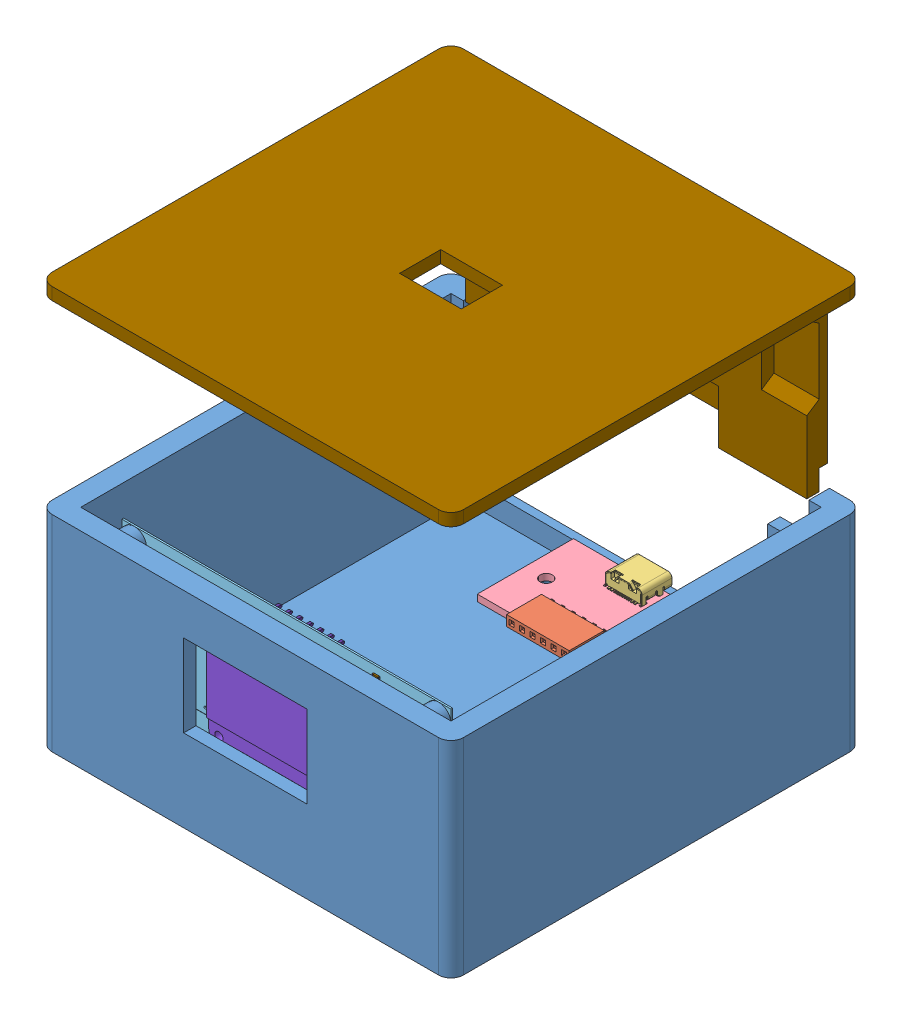
SolidWorks assembly 提醒喝水器, configuration 默认. Lengths in mm. (continued)
Components (placement in the parent): (continued)
- MainBoard-1: MainBoard [默认] at (-130.6896 -38.7345 40) size (80 40 10.66) (continued)
  - MainBoard(2)^MainBoard-1: MainBoard(2)^MainBoard [默认] at origin size (80 40 10.66) (virtual) (continued)
    - D2^MainBoard(2)_MainBoard-1: D2^MainBoard(2)_MainBoard [默认] at origin size (1.6 0.8 0.61) (virtual) (continued)
      - LED_0603-R^D2_MainBoard(2)_MainBoard-1: LED_0603-R^D2_MainBoard(2)_MainBoard [默认] at (39.878 9.398 0) x (-1 0 0) z (0 0 1) size (1.6 0.8 0.47) (virtual) (continued)
        - LED_0603-R-6878_AF0_ASM^LED_0603-R_D2_MainBoard(2)_MainBoard-1: LED_0603-R-6878_AF0_ASM^LED_0603-R_D2_MainBoard(2)_MainBoard [默认] at origin size (1.6 0.8 0.47) (virtual)
          - LED_0603-R-4157_AF0_ASM^LED_0603-R-6878_AF0_ASM_LED_0603-R_D2_MainBoard(2)_MainBoard-1: LED_0603-R-4157_AF0_ASM^LED_0603-R-6878_AF0_ASM_LED_0603-R_D2_MainBoard(2)_MainBoard [默认] at origin size (1.6 0.8 0.47) (virtual)
            - _2_1_20001^LED_0603-R-4157_AF0_ASM_LED_0603-R-6878_AF0_ASM_LED_0603-R_D2_MainBoard(2)_MainBoard-1: _2_1_20001^LED_0603-R-4157_AF0_ASM_LED_0603-R-6878_AF0_ASM_LED_0603-R_D2_MainBoard(2)_MainBoard [默认] at origin size (0.2 0.8 0.2) (virtual)
            - _5_2__1_20001^LED_0603-R-4157_AF0_ASM_LED_0603-R-6878_AF0_ASM_LED_0603-R_D2_MainBoard(2)_MainBoard-1: _5_2__1_20001^LED_0603-R-4157_AF0_ASM_LED_0603-R-6878_AF0_ASM_LED_0603-R_D2_MainBoard(2)_MainBoard [默认] at origin size (0.31 0.14 0) (virtual)
            - 4_1_200^LED_0603-R-4157_AF0_ASM_LED_0603-R-6878_AF0_ASM_LED_0603-R_D2_MainBoard(2)_MainBoard-1: 4_1_200^LED_0603-R-4157_AF0_ASM_LED_0603-R-6878_AF0_ASM_LED_0603-R_D2_MainBoard(2)_MainBoard [默认] at origin size (0.2 0.8 0.2) (virtual)
            - _5_1__1_20001^LED_0603-R-4157_AF0_ASM_LED_0603-R-6878_AF0_ASM_LED_0603-R_D2_MainBoard(2)_MainBoard-1: _5_1__1_20001^LED_0603-R-4157_AF0_ASM_LED_0603-R-6878_AF0_ASM_LED_0603-R_D2_MainBoard(2)_MainBoard [默认] at origin size (0.31 0.14 0) (virtual)
            - 1_1_2_3_4_5_6_7_8_000^LED_0603-R-4157_AF0_ASM_LED_0603-R-6878_AF0_ASM_LED_0603-R_D2_MainBoard(2)_MainBoard-1: 1_1_2_3_4_5_6_7_8_000^LED_0603-R-4157_AF0_ASM_LED_0603-R-6878_AF0_ASM_LED_0603-R_D2_MainBoard(2)_MainBoard [默认] at origin size (1.6 0.8 0.47) (virtual)
      - LED_0603______^D2_MainBoard(2)_MainBoard-1: LED_0603______^D2_MainBoard(2)_MainBoard [默认] at (39.878 9.398 0) x (1 0 0) z (0 0 1) size (1.2 0.8 0.4) (virtual)
    - D1^MainBoard(2)_MainBoard-1: D1^MainBoard(2)_MainBoard [默认] at origin size (1.5 3.4 1.5) (virtual)
      - MINI-MELF^D1_MainBoard(2)_MainBoard-1: MINI-MELF^D1_MainBoard(2)_MainBoard [默认] at (43.6879 20.0661 0) x (0 -1 0) z (0 0 1) size (3.4 1.5 1.5) (virtual)
        - MINI-MELF-5^MINI-MELF_D1_MainBoard(2)_MainBoard-1: MINI-MELF-5^MINI-MELF_D1_MainBoard(2)_MainBoard [默认] at origin size (3.4 1.5 1.5) (virtual)
        - LOGO______.____^MINI-MELF_D1_MainBoard(2)_MainBoard-1: LOGO______.____^MINI-MELF_D1_MainBoard(2)_MainBoard [默认] at (0.0006 0.0003 0.0498) x (-1 0 0) z (0 0 -1) size (0.06 0.07 0) (virtual)
    - C9^MainBoard(2)_MainBoard-1: C9^MainBoard(2)_MainBoard [默认] at origin size (1.22 2 0.52) (virtual)
      - c_0805^C9_MainBoard(2)_MainBoard-1: c_0805^C9_MainBoard(2)_MainBoard [默认] at (51.4351 17.1449 0) x (0 -1 0) z (0 0 1) size (2 1.22 0.52) (virtual)
        - C_0805-3038_AF0_ASM^c_0805_C9_MainBoard(2)_MainBoard-1: C_0805-3038_AF0_ASM^c_0805_C9_MainBoard(2)_MainBoard [默认] at origin size (2 1.22 0.52) (virtual)
          - C_0805-10418_AF0_ASM^C_0805-3038_AF0_ASM_c_0805_C9_MainBoard(2)_MainBoard-1: C_0805-10418_AF0_ASM^C_0805-3038_AF0_ASM_c_0805_C9_MainBoard(2)_MainBoard [默认] at origin size (2 1.22 0.52) (virtual)
            - 500^C_0805-10418_AF0_ASM_C_0805-3038_AF0_ASM_c_0805_C9_MainBoard(2)_MainBoard-1: 500^C_0805-10418_AF0_ASM_C_0805-3038_AF0_ASM_c_0805_C9_MainBoard(2)_MainBoard [默认] at origin size (0.3 1.22 0.52) (virtual)
            - _1_1_2_3_4_5_6_AF0^C_0805-10418_AF0_ASM_C_0805-3038_AF0_ASM_c_0805_C9_MainBoard(2)_MainBoard-1: _1_1_2_3_4_5_6_AF0^C_0805-10418_AF0_ASM_C_0805-3038_AF0_ASM_c_0805_C9_MainBoard(2)_MainBoard [默认] at origin size (1.4 1.2 0.5) (virtual)
            - 400^C_0805-10418_AF0_ASM_C_0805-3038_AF0_ASM_c_0805_C9_MainBoard(2)_MainBoard-1: 400^C_0805-10418_AF0_ASM_C_0805-3038_AF0_ASM_c_0805_C9_MainBoard(2)_MainBoard [默认] at origin size (0.3 1.22 0.52) (virtual)
    - C8^MainBoard(2)_MainBoard-1: C8^MainBoard(2)_MainBoard [默认] at origin size (2 1.22 0.52) (virtual)
      - c_0805^C8_MainBoard(2)_MainBoard-1: c_0805^C8_MainBoard(2)_MainBoard [默认] at (58.5469 12.1919 0) x (-1 0 0) z (0 0 1) size (2 1.22 0.52) (virtual)
        - C_0805-3038_AF0_ASM^c_0805_C8_MainBoard(2)_MainBoard-1: C_0805-3038_AF0_ASM^c_0805_C8_MainBoard(2)_MainBoard [默认] at origin size (2 1.22 0.52) (virtual)
          - C_0805-10418_AF0_ASM^C_0805-3038_AF0_ASM_c_0805_C8_MainBoard(2)_MainBoard-1: C_0805-10418_AF0_ASM^C_0805-3038_AF0_ASM_c_0805_C8_MainBoard(2)_MainBoard [默认] at origin size (2 1.22 0.52) (virtual)
            - 500^C_0805-10418_AF0_ASM_C_0805-3038_AF0_ASM_c_0805_C8_MainBoard(2)_MainBoard-1: 500^C_0805-10418_AF0_ASM_C_0805-3038_AF0_ASM_c_0805_C8_MainBoard(2)_MainBoard [默认] at origin size (0.3 1.22 0.52) (virtual)
            - _1_1_2_3_4_5_6_AF0^C_0805-10418_AF0_ASM_C_0805-3038_AF0_ASM_c_0805_C8_MainBoard(2)_MainBoard-1: _1_1_2_3_4_5_6_AF0^C_0805-10418_AF0_ASM_C_0805-3038_AF0_ASM_c_0805_C8_MainBoard(2)_MainBoard [默认] at origin size (1.4 1.2 0.5) (virtual)
            - 400^C_0805-10418_AF0_ASM_C_0805-3038_AF0_ASM_c_0805_C8_MainBoard(2)_MainBoard-1: 400^C_0805-10418_AF0_ASM_C_0805-3038_AF0_ASM_c_0805_C8_MainBoard(2)_MainBoard [默认] at origin size (0.3 1.22 0.52) (virtual)
    - C7^MainBoard(2)_MainBoard-1: C7^MainBoard(2)_MainBoard [默认] at origin size (1.6 0.82 0.82) (virtual)
      - c_0603^C7_MainBoard(2)_MainBoard-1: c_0603^C7_MainBoard(2)_MainBoard [默认] at (55.4989 19.431 0) x (-1 0 0) z (0 0 1) size (1.6 0.82 0.82) (virtual)
        - C_0603-7177_AF0_ASM^c_0603_C7_MainBoard(2)_MainBoard-1: C_0603-7177_AF0_ASM^c_0603_C7_MainBoard(2)_MainBoard [默认] at origin size (1.6 0.82 0.82) (virtual)
          - C_0603-683_AF0_ASM^C_0603-7177_AF0_ASM_c_0603_C7_MainBoard(2)_MainBoard-1: C_0603-683_AF0_ASM^C_0603-7177_AF0_ASM_c_0603_C7_MainBoard(2)_MainBoard [默认] at origin size (1.6 0.82 0.82) (virtual)
            - 2_1_200^C_0603-683_AF0_ASM_C_0603-7177_AF0_ASM_c_0603_C7_MainBoard(2)_MainBoard-1: 2_1_200^C_0603-683_AF0_ASM_C_0603-7177_AF0_ASM_c_0603_C7_MainBoard(2)_MainBoard [默认] at origin size (0.3 0.82 0.82) (virtual)
            - _1_1_2_3_4_5_AF0^C_0603-683_AF0_ASM_C_0603-7177_AF0_ASM_c_0603_C7_MainBoard(2)_MainBoard-1: _1_1_2_3_4_5_AF0^C_0603-683_AF0_ASM_C_0603-7177_AF0_ASM_c_0603_C7_MainBoard(2)_MainBoard [默认] at origin size (1 0.8 0.8) (virtual)
            - 3_1_200^C_0603-683_AF0_ASM_C_0603-7177_AF0_ASM_c_0603_C7_MainBoard(2)_MainBoard-1: 3_1_200^C_0603-683_AF0_ASM_C_0603-7177_AF0_ASM_c_0603_C7_MainBoard(2)_MainBoard [默认] at origin size (0.3 0.82 0.82) (virtual)
    - C6^MainBoard(2)_MainBoard-1: C6^MainBoard(2)_MainBoard [默认] at origin size (1.6 0.82 0.82) (virtual)
      - c_0603^C6_MainBoard(2)_MainBoard-1: c_0603^C6_MainBoard(2)_MainBoard [默认] at (73.6601 26.289 0) x (1 0 0) z (0 0 1) size (1.6 0.82 0.82) (virtual)
        - C_0603-7177_AF0_ASM^c_0603_C6_MainBoard(2)_MainBoard-1: C_0603-7177_AF0_ASM^c_0603_C6_MainBoard(2)_MainBoard [默认] at origin size (1.6 0.82 0.82) (virtual)
          - C_0603-683_AF0_ASM^C_0603-7177_AF0_ASM_c_0603_C6_MainBoard(2)_MainBoard-1: C_0603-683_AF0_ASM^C_0603-7177_AF0_ASM_c_0603_C6_MainBoard(2)_MainBoard [默认] at origin size (1.6 0.82 0.82) (virtual)
            - 2_1_200^C_0603-683_AF0_ASM_C_0603-7177_AF0_ASM_c_0603_C6_MainBoard(2)_MainBoard-1: 2_1_200^C_0603-683_AF0_ASM_C_0603-7177_AF0_ASM_c_0603_C6_MainBoard(2)_MainBoard [默认] at origin size (0.3 0.82 0.82) (virtual)
            - _1_1_2_3_4_5_AF0^C_0603-683_AF0_ASM_C_0603-7177_AF0_ASM_c_0603_C6_MainBoard(2)_MainBoard-1: _1_1_2_3_4_5_AF0^C_0603-683_AF0_ASM_C_0603-7177_AF0_ASM_c_0603_C6_MainBoard(2)_MainBoard [默认] at origin size (1 0.8 0.8) (virtual)
            - 3_1_200^C_0603-683_AF0_ASM_C_0603-7177_AF0_ASM_c_0603_C6_MainBoard(2)_MainBoard-1: 3_1_200^C_0603-683_AF0_ASM_C_0603-7177_AF0_ASM_c_0603_C6_MainBoard(2)_MainBoard [默认] at origin size (0.3 0.82 0.82) (virtual)
    - C5^MainBoard(2)_MainBoard-1: C5^MainBoard(2)_MainBoard [默认] at origin size (1.6 0.82 0.82) (virtual)
      - c_0603^C5_MainBoard(2)_MainBoard-1: c_0603^C5_MainBoard(2)_MainBoard [默认] at (73.6599 32.766 0) x (-1 0 0) z (0 0 1) size (1.6 0.82 0.82) (virtual)
        - C_0603-7177_AF0_ASM^c_0603_C5_MainBoard(2)_MainBoard-1: C_0603-7177_AF0_ASM^c_0603_C5_MainBoard(2)_MainBoard [默认] at origin size (1.6 0.82 0.82) (virtual)
          - C_0603-683_AF0_ASM^C_0603-7177_AF0_ASM_c_0603_C5_MainBoard(2)_MainBoard-1: C_0603-683_AF0_ASM^C_0603-7177_AF0_ASM_c_0603_C5_MainBoard(2)_MainBoard [默认] at origin size (1.6 0.82 0.82) (virtual)
            - 2_1_200^C_0603-683_AF0_ASM_C_0603-7177_AF0_ASM_c_0603_C5_MainBoard(2)_MainBoard-1: 2_1_200^C_0603-683_AF0_ASM_C_0603-7177_AF0_ASM_c_0603_C5_MainBoard(2)_MainBoard [默认] at origin size (0.3 0.82 0.82) (virtual)
            - _1_1_2_3_4_5_AF0^C_0603-683_AF0_ASM_C_0603-7177_AF0_ASM_c_0603_C5_MainBoard(2)_MainBoard-1: _1_1_2_3_4_5_AF0^C_0603-683_AF0_ASM_C_0603-7177_AF0_ASM_c_0603_C5_MainBoard(2)_MainBoard [默认] at origin size (1 0.8 0.8) (virtual)
            - 3_1_200^C_0603-683_AF0_ASM_C_0603-7177_AF0_ASM_c_0603_C5_MainBoard(2)_MainBoard-1: 3_1_200^C_0603-683_AF0_ASM_C_0603-7177_AF0_ASM_c_0603_C5_MainBoard(2)_MainBoard [默认] at origin size (0.3 0.82 0.82) (virtual)
    - C4^MainBoard(2)_MainBoard-1: C4^MainBoard(2)_MainBoard [默认] at origin size (0.82 1.6 0.82) (virtual)
      - c_0603^C4_MainBoard(2)_MainBoard-1: c_0603^C4_MainBoard(2)_MainBoard [默认] at (12.192 7.6201 0) x (0 1 0) z (0 0 1) size (1.6 0.82 0.82) (virtual)
        - C_0603-7177_AF0_ASM^c_0603_C4_MainBoard(2)_MainBoard-1: C_0603-7177_AF0_ASM^c_0603_C4_MainBoard(2)_MainBoard [默认] at origin size (1.6 0.82 0.82) (virtual)
          - C_0603-683_AF0_ASM^C_0603-7177_AF0_ASM_c_0603_C4_MainBoard(2)_MainBoard-1: C_0603-683_AF0_ASM^C_0603-7177_AF0_ASM_c_0603_C4_MainBoard(2)_MainBoard [默认] at origin size (1.6 0.82 0.82) (virtual)
            - 2_1_200^C_0603-683_AF0_ASM_C_0603-7177_AF0_ASM_c_0603_C4_MainBoard(2)_MainBoard-1: 2_1_200^C_0603-683_AF0_ASM_C_0603-7177_AF0_ASM_c_0603_C4_MainBoard(2)_MainBoard [默认] at origin size (0.3 0.82 0.82) (virtual)
            - _1_1_2_3_4_5_AF0^C_0603-683_AF0_ASM_C_0603-7177_AF0_ASM_c_0603_C4_MainBoard(2)_MainBoard-1: _1_1_2_3_4_5_AF0^C_0603-683_AF0_ASM_C_0603-7177_AF0_ASM_c_0603_C4_MainBoard(2)_MainBoard [默认] at origin size (1 0.8 0.8) (virtual)
            - 3_1_200^C_0603-683_AF0_ASM_C_0603-7177_AF0_ASM_c_0603_C4_MainBoard(2)_MainBoard-1: 3_1_200^C_0603-683_AF0_ASM_C_0603-7177_AF0_ASM_c_0603_C4_MainBoard(2)_MainBoard [默认] at origin size (0.3 0.82 0.82) (virtual)
    - C3^MainBoard(2)_MainBoard-1: C3^MainBoard(2)_MainBoard [默认] at origin size (0.82 1.6 0.82) (virtual)
      - c_0603^C3_MainBoard(2)_MainBoard-1: c_0603^C3_MainBoard(2)_MainBoard [默认] at (59.8169 31.3542 0) x (0 1 0) z (0 0 1) size (1.6 0.82 0.82) (virtual)
        - C_0603-7177_AF0_ASM^c_0603_C3_MainBoard(2)_MainBoard-1: C_0603-7177_AF0_ASM^c_0603_C3_MainBoard(2)_MainBoard [默认] at origin size (1.6 0.82 0.82) (virtual)
          - C_0603-683_AF0_ASM^C_0603-7177_AF0_ASM_c_0603_C3_MainBoard(2)_MainBoard-1: C_0603-683_AF0_ASM^C_0603-7177_AF0_ASM_c_0603_C3_MainBoard(2)_MainBoard [默认] at origin size (1.6 0.82 0.82) (virtual)
            - 2_1_200^C_0603-683_AF0_ASM_C_0603-7177_AF0_ASM_c_0603_C3_MainBoard(2)_MainBoard-1: 2_1_200^C_0603-683_AF0_ASM_C_0603-7177_AF0_ASM_c_0603_C3_MainBoard(2)_MainBoard [默认] at origin size (0.3 0.82 0.82) (virtual)
            - _1_1_2_3_4_5_AF0^C_0603-683_AF0_ASM_C_0603-7177_AF0_ASM_c_0603_C3_MainBoard(2)_MainBoard-1: _1_1_2_3_4_5_AF0^C_0603-683_AF0_ASM_C_0603-7177_AF0_ASM_c_0603_C3_MainBoard(2)_MainBoard [默认] at origin size (1 0.8 0.8) (virtual)
            - 3_1_200^C_0603-683_AF0_ASM_C_0603-7177_AF0_ASM_c_0603_C3_MainBoard(2)_MainBoard-1: 3_1_200^C_0603-683_AF0_ASM_C_0603-7177_AF0_ASM_c_0603_C3_MainBoard(2)_MainBoard [默认] at origin size (0.3 0.82 0.82) (virtual)
    - C2^MainBoard(2)_MainBoard-1: C2^MainBoard(2)_MainBoard [默认] at origin size (0.82 1.6 0.82) (virtual)
      - c_0603^C2_MainBoard(2)_MainBoard-1: c_0603^C2_MainBoard(2)_MainBoard [默认] at (45.3389 3.2872 0) x (0 1 0) z (0 0 1) size (1.6 0.82 0.82) (virtual)
        - C_0603-7177_AF0_ASM^c_0603_C2_MainBoard(2)_MainBoard-1: C_0603-7177_AF0_ASM^c_0603_C2_MainBoard(2)_MainBoard [默认] at origin size (1.6 0.82 0.82) (virtual)
          - C_0603-683_AF0_ASM^C_0603-7177_AF0_ASM_c_0603_C2_MainBoard(2)_MainBoard-1: C_0603-683_AF0_ASM^C_0603-7177_AF0_ASM_c_0603_C2_MainBoard(2)_MainBoard [默认] at origin size (1.6 0.82 0.82) (virtual)
            - 2_1_200^C_0603-683_AF0_ASM_C_0603-7177_AF0_ASM_c_0603_C2_MainBoard(2)_MainBoard-1: 2_1_200^C_0603-683_AF0_ASM_C_0603-7177_AF0_ASM_c_0603_C2_MainBoard(2)_MainBoard [默认] at origin size (0.3 0.82 0.82) (virtual)
            - _1_1_2_3_4_5_AF0^C_0603-683_AF0_ASM_C_0603-7177_AF0_ASM_c_0603_C2_MainBoard(2)_MainBoard-1: _1_1_2_3_4_5_AF0^C_0603-683_AF0_ASM_C_0603-7177_AF0_ASM_c_0603_C2_MainBoard(2)_MainBoard [默认] at origin size (1 0.8 0.8) (virtual)
            - 3_1_200^C_0603-683_AF0_ASM_C_0603-7177_AF0_ASM_c_0603_C2_MainBoard(2)_MainBoard-1: 3_1_200^C_0603-683_AF0_ASM_C_0603-7177_AF0_ASM_c_0603_C2_MainBoard(2)_MainBoard [默认] at origin size (0.3 0.82 0.82) (virtual)
    - C1^MainBoard(2)_MainBoard-1: C1^MainBoard(2)_MainBoard [默认] at origin size (0.82 1.6 0.82) (virtual)
      - c_0603^C1_MainBoard(2)_MainBoard-1: c_0603^C1_MainBoard(2)_MainBoard [默认] at (8.89 7.6199 0) x (0 -1 0) z (0 0 1) size (1.6 0.82 0.82) (virtual)
        - C_0603-7177_AF0_ASM^c_0603_C1_MainBoard(2)_MainBoard-1: C_0603-7177_AF0_ASM^c_0603_C1_MainBoard(2)_MainBoard [默认] at origin size (1.6 0.82 0.82) (virtual)
          - C_0603-683_AF0_ASM^C_0603-7177_AF0_ASM_c_0603_C1_MainBoard(2)_MainBoard-1: C_0603-683_AF0_ASM^C_0603-7177_AF0_ASM_c_0603_C1_MainBoard(2)_MainBoard [默认] at origin size (1.6 0.82 0.82) (virtual)
            - 2_1_200^C_0603-683_AF0_ASM_C_0603-7177_AF0_ASM_c_0603_C1_MainBoard(2)_MainBoard-1: 2_1_200^C_0603-683_AF0_ASM_C_0603-7177_AF0_ASM_c_0603_C1_MainBoard(2)_MainBoard [默认] at origin size (0.3 0.82 0.82) (virtual)
            - _1_1_2_3_4_5_AF0^C_0603-683_AF0_ASM_C_0603-7177_AF0_ASM_c_0603_C1_MainBoard(2)_MainBoard-1: _1_1_2_3_4_5_AF0^C_0603-683_AF0_ASM_C_0603-7177_AF0_ASM_c_0603_C1_MainBoard(2)_MainBoard [默认] at origin size (1 0.8 0.8) (virtual)
            - 3_1_200^C_0603-683_AF0_ASM_C_0603-7177_AF0_ASM_c_0603_C1_MainBoard(2)_MainBoard-1: 3_1_200^C_0603-683_AF0_ASM_C_0603-7177_AF0_ASM_c_0603_C1_MainBoard(2)_MainBoard [默认] at origin size (0.3 0.82 0.82) (virtual)
- OLED-1: OLED [默认] at (-75.4466 -2.0805 44.1) x (-1 0 0) z (0 0 -1) size (29.97 28.97 13.2)
  - 3D_PCB_7针SPI_2022-02-05_2022-02-05(2)^OLED-1: 3D_PCB_7针SPI_2022-02-05_2022-02-05(2)^OLED [默认] at origin size (29.97 28.97 13.2) (virtual)
    - R5(2)^3D_PCB_7针SPI_2022-02-05_2022-02-05(2)_OLED-1: R5(2)^3D_PCB_7针SPI_2022-02-05_2022-02-05(2)_OLED [默认] at (11.176 -11.303 1.6) x (0 -1 0) z (0 0 1) size (1.6 0.8 0.8) (virtual)
      - R0603^R5(2)_3D_PCB_7针SPI_2022-02-05_2022-02-05(2)_OLED-1: R0603^R5(2)_3D_PCB_7针SPI_2022-02-05_2022-02-05(2)_OLED [默认] at origin size (1.6 0.8 0.8) (virtual)
        - =_[0_1_1_5]^R0603_R5(2)_3D_PCB_7针SPI_2022-02-05_2022-02-05(2)_OLED-1: =_[0_1_1_5]^R0603_R5(2)_3D_PCB_7针SPI_2022-02-05_2022-02-05(2)_OLED [默认] at (0 0 0.4) size (1.6 0.8 0.8) (virtual)
    - R6(2)^3D_PCB_7针SPI_2022-02-05_2022-02-05(2)_OLED-1: R6(2)^3D_PCB_7针SPI_2022-02-05_2022-02-05(2)_OLED [默认] at (25.5271 -6.985 1.6) x (-1 0 0) z (0 0 1) size (1.6 0.8 0.8) (virtual)
      - R0603^R6(2)_3D_PCB_7针SPI_2022-02-05_2022-02-05(2)_OLED-1: R0603^R6(2)_3D_PCB_7针SPI_2022-02-05_2022-02-05(2)_OLED [默认] at origin size (1.6 0.8 0.8) (virtual)
        - =_[0_1_1_5]^R0603_R6(2)_3D_PCB_7针SPI_2022-02-05_2022-02-05(2)_OLED-1: =_[0_1_1_5]^R0603_R6(2)_3D_PCB_7针SPI_2022-02-05_2022-02-05(2)_OLED [默认] at (0 0 0.4) size (1.6 0.8 0.8) (virtual)
    - J1^3D_PCB_7针SPI_2022-02-05_2022-02-05(2)_OLED-1: J1^3D_PCB_7针SPI_2022-02-05_2022-02-05(2)_OLED [默认] at (15.113 -1.524 1.6) size (17.53 2.5 11.6) (virtual)
      - HDR-M-2.54_1X7^J1_3D_PCB_7针SPI_2022-02-05_2022-02-05(2)_OLED-1: HDR-M-2.54_1X7^J1_3D_PCB_7针SPI_2022-02-05_2022-02-05(2)_OLED [默认] at origin size (17.53 2.5 11.6) (virtual)
        - =_[0_1_1_10]^HDR-M-2.54_1X7_J1_3D_PCB_7针SPI_2022-02-05_2022-02-05(2)_OLED-1: =_[0_1_1_10]^HDR-M-2.54_1X7_J1_3D_PCB_7针SPI_2022-02-05_2022-02-05(2)_OLED [默认] at origin size (17.53 2.5 11.6) (virtual)
    - C5(2)^3D_PCB_7针SPI_2022-02-05_2022-02-05(2)_OLED-1: C5(2)^3D_PCB_7针SPI_2022-02-05_2022-02-05(2)_OLED [默认] at (9.271 -11.303 1.6) x (0 -1 0) z (0 0 1) size (1.6 0.8 0.8) (virtual)
      - C0603^C5(2)_3D_PCB_7针SPI_2022-02-05_2022-02-05(2)_OLED-1: C0603^C5(2)_3D_PCB_7针SPI_2022-02-05_2022-02-05(2)_OLED [默认] at origin size (1.6 0.8 0.8) (virtual)
        - =_[0_1_1_14]^C0603_C5(2)_3D_PCB_7针SPI_2022-02-05_2022-02-05(2)_OLED-1: =_[0_1_1_14]^C0603_C5(2)_3D_PCB_7针SPI_2022-02-05_2022-02-05(2)_OLED [默认] at (0 0 0.4) size (1.6 0.8 0.8) (virtual)
    - C2(2)^3D_PCB_7针SPI_2022-02-05_2022-02-05(2)_OLED-1: C2(2)^3D_PCB_7针SPI_2022-02-05_2022-02-05(2)_OLED [默认] at (24.257 -11.176 1.6) x (0 -1 0) z (0 0 1) size (1.6 0.8 0.8) (virtual)
      - C0603^C2(2)_3D_PCB_7针SPI_2022-02-05_2022-02-05(2)_OLED-1: C0603^C2(2)_3D_PCB_7针SPI_2022-02-05_2022-02-05(2)_OLED [默认] at origin size (1.6 0.8 0.8) (virtual)
        - =_[0_1_1_14]^C0603_C2(2)_3D_PCB_7针SPI_2022-02-05_2022-02-05(2)_OLED-1: =_[0_1_1_14]^C0603_C2(2)_3D_PCB_7针SPI_2022-02-05_2022-02-05(2)_OLED [默认] at (0 0 0.4) size (1.6 0.8 0.8) (virtual)
    - C3(2)^3D_PCB_7针SPI_2022-02-05_2022-02-05(2)_OLED-1: C3(2)^3D_PCB_7针SPI_2022-02-05_2022-02-05(2)_OLED [默认] at (19.558 -11.176 1.6) x (0 1 0) z (0 0 1) size (1.6 0.8 0.8) (virtual)
      - C0603^C3(2)_3D_PCB_7针SPI_2022-02-05_2022-02-05(2)_OLED-1: C0603^C3(2)_3D_PCB_7针SPI_2022-02-05_2022-02-05(2)_OLED [默认] at origin size (1.6 0.8 0.8) (virtual)
        - =_[0_1_1_14]^C0603_C3(2)_3D_PCB_7针SPI_2022-02-05_2022-02-05(2)_OLED-1: =_[0_1_1_14]^C0603_C3(2)_3D_PCB_7针SPI_2022-02-05_2022-02-05(2)_OLED [默认] at (0 0 0.4) size (1.6 0.8 0.8) (virtual)
    - C4(2)^3D_PCB_7针SPI_2022-02-05_2022-02-05(2)_OLED-1: C4(2)^3D_PCB_7针SPI_2022-02-05_2022-02-05(2)_OLED [默认] at (21.463 -11.176 1.6) x (0 1 0) z (0 0 1) size (1.6 0.8 0.8) (virtual)
      - C0603^C4(2)_3D_PCB_7针SPI_2022-02-05_2022-02-05(2)_OLED-1: C0603^C4(2)_3D_PCB_7针SPI_2022-02-05_2022-02-05(2)_OLED [默认] at origin size (1.6 0.8 0.8) (virtual)
        - =_[0_1_1_14]^C0603_C4(2)_3D_PCB_7针SPI_2022-02-05_2022-02-05(2)_OLED-1: =_[0_1_1_14]^C0603_C4(2)_3D_PCB_7针SPI_2022-02-05_2022-02-05(2)_OLED [默认] at (0 0 0.4) size (1.6 0.8 0.8) (virtual)
    - C7(2)^3D_PCB_7针SPI_2022-02-05_2022-02-05(2)_OLED-1: C7(2)^3D_PCB_7针SPI_2022-02-05_2022-02-05(2)_OLED [默认] at (18.923 -5.461 1.6) x (0 -1 0) z (0 0 1) size (1.6 0.8 0.8) (virtual)
      - C0603^C7(2)_3D_PCB_7针SPI_2022-02-05_2022-02-05(2)_OLED-1: C0603^C7(2)_3D_PCB_7针SPI_2022-02-05_2022-02-05(2)_OLED [默认] at origin size (1.6 0.8 0.8) (virtual)
        - =_[0_1_1_14]^C0603_C7(2)_3D_PCB_7针SPI_2022-02-05_2022-02-05(2)_OLED-1: =_[0_1_1_14]^C0603_C7(2)_3D_PCB_7针SPI_2022-02-05_2022-02-05(2)_OLED [默认] at (0 0 0.4) size (1.6 0.8 0.8) (virtual)
    - C1(2)^3D_PCB_7针SPI_2022-02-05_2022-02-05(2)_OLED-1: C1(2)^3D_PCB_7针SPI_2022-02-05_2022-02-05(2)_OLED [默认] at (26.5431 -11.176 1.6) x (0 -1 0) z (0 0 1) size (1.6 0.8 0.8) (virtual)
      - C0603^C1(2)_3D_PCB_7针SPI_2022-02-05_2022-02-05(2)_OLED-1: C0603^C1(2)_3D_PCB_7针SPI_2022-02-05_2022-02-05(2)_OLED [默认] at origin size (1.6 0.8 0.8) (virtual)
        - =_[0_1_1_14]^C0603_C1(2)_3D_PCB_7针SPI_2022-02-05_2022-02-05(2)_OLED-1: =_[0_1_1_14]^C0603_C1(2)_3D_PCB_7针SPI_2022-02-05_2022-02-05(2)_OLED [默认] at (0 0 0.4) size (1.6 0.8 0.8) (virtual)
    - C6(2)^3D_PCB_7针SPI_2022-02-05_2022-02-05(2)_OLED-1: C6(2)^3D_PCB_7针SPI_2022-02-05_2022-02-05(2)_OLED [默认] at (7.366 -11.303 1.6) x (0 -1 0) z (0 0 1) size (1.6 0.8 0.8) (virtual)
      - C0603^C6(2)_3D_PCB_7针SPI_2022-02-05_2022-02-05(2)_OLED-1: C0603^C6(2)_3D_PCB_7针SPI_2022-02-05_2022-02-05(2)_OLED [默认] at origin size (1.6 0.8 0.8) (virtual)
        - =_[0_1_1_14]^C0603_C6(2)_3D_PCB_7针SPI_2022-02-05_2022-02-05(2)_OLED-1: =_[0_1_1_14]^C0603_C6(2)_3D_PCB_7针SPI_2022-02-05_2022-02-05(2)_OLED [默认] at (0 0 0.4) size (1.6 0.8 0.8) (virtual)
    - U1(2)^3D_PCB_7针SPI_2022-02-05_2022-02-05(2)_OLED-1: U1(2)^3D_PCB_7针SPI_2022-02-05_2022-02-05(2)_OLED [默认] at (21.844 -5.842 1.6) x (0 -1 0) z (0 0 1) size (2.5 2.89 1.05) (virtual)
      - SOT-23-3_L2.9-W1.3-P1.90-LS2.4-BR^U1(2)_3D_PCB_7针SPI_2022-02-05_2022-02-05(2)_OLED-1: SOT-23-3_L2.9-W1.3-P1.90-LS2.4-BR^U1(2)_3D_PCB_7针SPI_2022-02-05_2022-02-05(2)_OLED [默认] at origin size (2.5 2.89 1.05) (virtual)
        - COMPOUND(2)^SOT-23-3_L2.9-W1.3-P1.90-LS2.4-BR_U1(2)_3D_PCB_7针SPI_2022-02-05_2022-02-05(2)_OLED-1: COMPOUND(2)^SOT-23-3_L2.9-W1.3-P1.90-LS2.4-BR_U1(2)_3D_PCB_7针SPI_2022-02-05_2022-02-05(2)_OLED [默认] at origin size (2.5 2.89 1.05) (virtual)
    - COMPOUND-0^3D_PCB_7针SPI_2022-02-05_2022-02-05(2)_OLED-1: COMPOUND-0^3D_PCB_7针SPI_2022-02-05_2022-02-05(2)_OLED [默认] at origin size (29.97 28.97 4.6) (virtual)
- 上盖-1: 上盖 [默认] at (-140.6896 48.7655 50) size (100 48 100)
Mates (geometry in assembly coordinates):
- 重合1: coincident anti-aligned: plane of 外壳-1 through (-103.5021 -37.2345 -36) normal (0 1 0); plane of Type-C_Ext-1/Type-C_Ext(2)^Type-C_Ext-1/Type-C_Ext PCB^Type-C_Ext(2)_Type-C_Ext-1 through (-90.7041 -37.2345 -36) normal (0 -1 0)
- 平行1: parallel aligned: plane of 外壳-1 through (-135.6896 -41.2345 -45) normal (0 0 1); plane of Type-C_Ext-1/Type-C_Ext(2)^Type-C_Ext-1/Type-C_Ext PCB^Type-C_Ext(2)_Type-C_Ext-1 through (-108.6111 -37.2345 -24.316) normal (0 0 1)
- 同心1: concentric aligned: circle of 外壳-1; circle of Type-C_Ext-1/Type-C_Ext(2)^Type-C_Ext-1/Type-C_Ext PCB^Type-C_Ext(2)_Type-C_Ext-1
- 平行2: parallel anti-aligned: plane of MainBoard-1/MainBoard(2)^MainBoard-1/Board^MainBoard(2)_MainBoard-1/Open CASCADE STEP translator 6.8 1.1.1^Board_MainBoard(2)_MainBoard-1 through (-130.6896 -38.7345 40) normal (0 0 1); plane of OLED-1/3D_PCB_7针SPI_2022-02-05_2022-02-05(2)^OLED-1/COMPOUND-0^3D_PCB_7针SPI_2022-02-05_2022-02-05(2)_OLED-1 through (-90.5084 -16.8409 42.5) normal (0 0 -1)
- 平行5: parallel aligned: plane of 外壳-1 through (-137.6896 3.7655 -50) normal (0 0 -1); plane of MainBoard-1/MainBoard(2)^MainBoard-1/Board^MainBoard(2)_MainBoard-1/Open CASCADE STEP translator 6.8 1.1.1^Board_MainBoard(2)_MainBoard-1 through (-130.6896 -38.7345 39.5885) normal (0 0 -1)
- 平行7: parallel aligned: plane of 外壳-1 through (-140.6896 -41.2345 50) normal (0 1 0); plane of MainBoard-1/MainBoard(2)^MainBoard-1/Board^MainBoard(2)_MainBoard-1/Open CASCADE STEP translator 6.8 1.1.1^Board_MainBoard(2)_MainBoard-1 through (-130.6896 1.2655 39.5885) normal (0 1 0)
- 重合13: coincident anti-aligned: plane of MainBoard-1/MainBoard(2)^MainBoard-1/Board^MainBoard(2)_MainBoard-1/Open CASCADE STEP translator 6.8 1.1.1^Board_MainBoard(2)_MainBoard-1 through (-130.6896 -38.7345 40) normal (0 0 1); plane of OLED-1/3D_PCB_7针SPI_2022-02-05_2022-02-05(2)^OLED-1/J1^3D_PCB_7针SPI_2022-02-05_2022-02-05(2)_OLED-1/HDR-M-2.54_1X7^J1_3D_PCB_7针SPI_2022-02-05_2022-02-05(2)_OLED-1/=_[0_1_1_10]^HDR-M-2.54_1X7_J1_3D_PCB_7针SPI_2022-02-05_2022-02-05(2)_OLED-1 through (-90.5596 -3.6045 40) normal (0 0 -1)
- 同心2: concentric anti-aligned: circle of 外壳-1; circle of MainBoard-1/MainBoard(2)^MainBoard-1/Board^MainBoard(2)_MainBoard-1/Open CASCADE STEP translator 6.8 1.1.1^Board_MainBoard(2)_MainBoard-1
- 重合14: coincident anti-aligned: plane of 外壳-1 through (-53.6896 -1.7345 40) normal (0 0 -1); plane of MainBoard-1/MainBoard(2)^MainBoard-1/Board^MainBoard(2)_MainBoard-1/Open CASCADE STEP translator 6.8 1.1.1^Board_MainBoard(2)_MainBoard-1 through (-130.6896 -38.7345 40) normal (0 0 1)
- 相切2: tangent: circle of MainBoard-1/MainBoard(2)^MainBoard-1/Board^MainBoard(2)_MainBoard-1/Open CASCADE STEP translator 6.8 1.1.1^Board_MainBoard(2)_MainBoard-1; plane of OLED-1/3D_PCB_7针SPI_2022-02-05_2022-02-05(2)^OLED-1/J1^3D_PCB_7针SPI_2022-02-05_2022-02-05(2)_OLED-1/HDR-M-2.54_1X7^J1_3D_PCB_7针SPI_2022-02-05_2022-02-05(2)_OLED-1/=_[0_1_1_10]^HDR-M-2.54_1X7_J1_3D_PCB_7针SPI_2022-02-05_2022-02-05(2)_OLED-1 through (-82.6196 -3.2845 45.3) normal (0 1 0)
- 平行8: parallel aligned: plane of MainBoard-1/MainBoard(2)^MainBoard-1/Board^MainBoard(2)_MainBoard-1/Open CASCADE STEP translator 6.8 1.1.1^Board_MainBoard(2)_MainBoard-1 through (-130.6896 1.2655 39.5885) normal (0 1 0); plane of OLED-1/3D_PCB_7针SPI_2022-02-05_2022-02-05(2)^OLED-1/J1^3D_PCB_7针SPI_2022-02-05_2022-02-05(2)_OLED-1/HDR-M-2.54_1X7^J1_3D_PCB_7针SPI_2022-02-05_2022-02-05(2)_OLED-1/=_[0_1_1_10]^HDR-M-2.54_1X7_J1_3D_PCB_7针SPI_2022-02-05_2022-02-05(2)_OLED-1 through (-82.6196 -3.2845 45.3) normal (0 1 0)
- 相切4: tangent: circle of MainBoard-1/MainBoard(2)^MainBoard-1/Board^MainBoard(2)_MainBoard-1/Open CASCADE STEP translator 6.8 1.1.1^Board_MainBoard(2)_MainBoard-1; plane of OLED-1/3D_PCB_7针SPI_2022-02-05_2022-02-05(2)^OLED-1/J1^3D_PCB_7针SPI_2022-02-05_2022-02-05(2)_OLED-1/HDR-M-2.54_1X7^J1_3D_PCB_7针SPI_2022-02-05_2022-02-05(2)_OLED-1/=_[0_1_1_10]^HDR-M-2.54_1X7_J1_3D_PCB_7针SPI_2022-02-05_2022-02-05(2)_OLED-1 through (-90.2396 -3.2845 45.3) normal (0 1 0)
- 相切5: tangent: circle of MainBoard-1/MainBoard(2)^MainBoard-1/Board^MainBoard(2)_MainBoard-1/Open CASCADE STEP translator 6.8 1.1.1^Board_MainBoard(2)_MainBoard-1; plane of OLED-1/3D_PCB_7针SPI_2022-02-05_2022-02-05(2)^OLED-1/J1^3D_PCB_7针SPI_2022-02-05_2022-02-05(2)_OLED-1/HDR-M-2.54_1X7^J1_3D_PCB_7针SPI_2022-02-05_2022-02-05(2)_OLED-1/=_[0_1_1_10]^HDR-M-2.54_1X7_J1_3D_PCB_7针SPI_2022-02-05_2022-02-05(2)_OLED-1 through (-90.2396 -3.6045 42.5) normal (1 0 0)
- 同心3: concentric: circle of 外壳-1; circle of 上盖-1
- 同心4: concentric aligned: circle of 外壳-1; circle of 上盖-1
